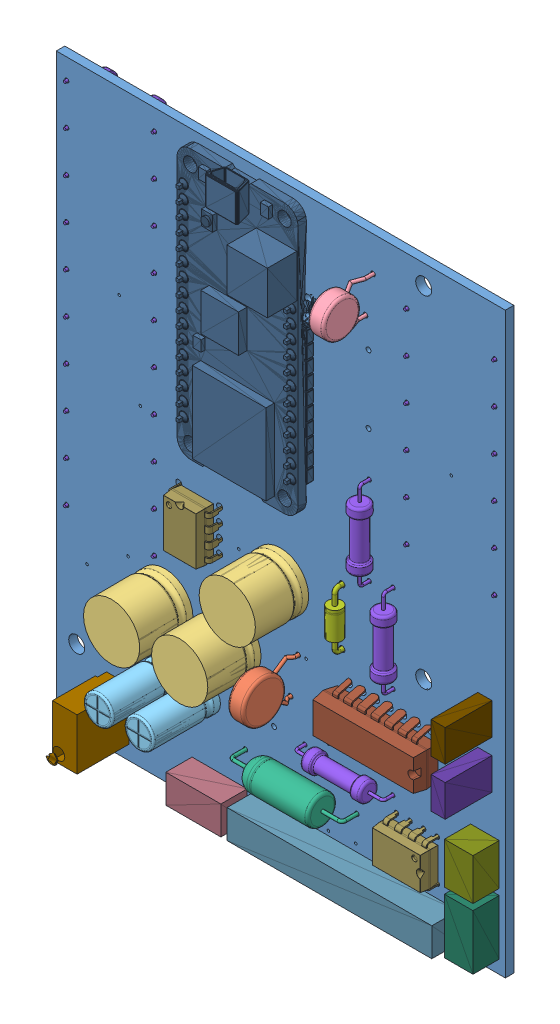
SolidWorks assembly MCB, configuration Default. Lengths in mm.
Overall size (83.82 111.16 36.76).
45 component instances, 18 part files, 0 mates.
Components (placement in the parent):
- SHEIKAHSLATE-1: SHEIKAHSLATE [Default] at origin size (83.82 111.16 36.76)
  - Board_SHEIKAHSLATE-1: Board_SHEIKAHSLATE [Default] at origin size (83.82 107.95 1.59)
  - HAU470KBAUARKR-1: HAU470KBAUARKR [Default] at (53.34 12.7 0.05) x (0 1 0) z (0 0 1) size (8 3 13.01)
  - MALREKA00DE433BG0K-1: MALREKA00DE433BG0K [Default] at (50.8 26.83 0.05) x (0 1 0) z (0 0 1) size (10.51 10.5 11.95)
  - MALREKA00DE433BG0K-2: MALREKA00DE433BG0K [Default] at (29.21 12.7 0.05) size (10.51 10.5 11.95)
  - MALREKA00DE433BG0K-3: MALREKA00DE433BG0K [Default] at (41.91 12.7 0.05) size (10.51 10.5 11.95)
  - A102J15C0GF5UAAP-1: A102J15C0GF5UAAP [Default] at (67.31 81.28 0.05) x (0 -1 0) z (0 0 1) size (7.99 3 12.01)
  - Noname_1-1: Noname_1 [Default] at (36.83 1.27 0.05) size (5.5 5.5 14.5)
  - Noname_1-2: Noname_1 [Default] at (29.21 1.27 0.05) size (5.5 5.5 14.5)
  - TVA1161-1: TVA1161 [Default] at (54.61 -3.81 0.05) size (21.4 5.51 7.51)
  - 1N5819G-1: 1N5819G [Default] at (62.23 26.67 0) x (0 -1 0) z (0 0 1) size (11.27 2.71 4.71)
  - Noname_2-1: Noname_2 [Default] at (67.31 43.18 0) x (0 -1 0) z (0 0 1) size (16.91 3.6 5.6)
  - Noname_2-2: Noname_2 [Default] at (46.99 58.42 -1.5896) x (0 1 0) z (0 0 -1) size (16.91 3.6 5.6)
  - Noname_2-3: Noname_2 [Default] at (19.05 87.63 -1.5896) x (-1 0 0) z (0 0 -1) size (16.91 3.6 5.6)
  - Noname_2-4: Noname_2 [Default] at (19.05 80.01 -1.5896) x (-1 0 0) z (0 0 -1) size (16.91 3.6 5.6)
  - Noname_2-5: Noname_2 [Default] at (19.05 72.39 -1.5896) x (-1 0 0) z (0 0 -1) size (16.91 3.6 5.6)
  - Noname_2-6: Noname_2 [Default] at (19.05 64.77 -1.5896) x (-1 0 0) z (0 0 -1) size (16.91 3.6 5.6)
  - Noname_2-7: Noname_2 [Default] at (19.05 57.15 -1.5896) x (-1 0 0) z (0 0 -1) size (16.91 3.6 5.6)
  - Noname_2-8: Noname_2 [Default] at (19.05 49.53 -1.5896) x (-1 0 0) z (0 0 -1) size (16.91 3.6 5.6)
  - Noname_2-9: Noname_2 [Default] at (19.05 41.91 -1.5896) x (-1 0 0) z (0 0 -1) size (16.91 3.6 5.6)
  - Noname_2-10: Noname_2 [Default] at (19.05 34.29 -1.5896) x (-1 0 0) z (0 0 -1) size (16.91 3.6 5.6)
  - Noname_2-11: Noname_2 [Default] at (19.05 26.67 -1.5896) x (-1 0 0) z (0 0 -1) size (16.91 3.6 5.6)
  - Noname_2-12: Noname_2 [Default] at (19.05 19.05 -1.5896) x (-1 0 0) z (0 0 -1) size (16.91 3.6 5.6)
  - Noname_2-13: Noname_2 [Default] at (82.55 44.45 -1.5896) x (1 0 0) z (0 0 -1) size (16.91 3.6 5.6)
  - Noname_2-14: Noname_2 [Default] at (82.55 52.07 -1.5896) x (1 0 0) z (0 0 -1) size (16.91 3.6 5.6)
  - Noname_2-15: Noname_2 [Default] at (82.55 59.69 -1.5896) x (1 0 0) z (0 0 -1) size (16.91 3.6 5.6)
  - Noname_2-16: Noname_2 [Default] at (82.55 67.31 -1.5896) x (1 0 0) z (0 0 -1) size (16.91 3.6 5.6)
  - Noname_2-17: Noname_2 [Default] at (82.55 74.93 -1.5896) x (1 0 0) z (0 0 -1) size (16.91 3.6 5.6)
  - Noname_2-18: Noname_2 [Default] at (82.55 82.55 -1.5896) x (1 0 0) z (0 0 -1) size (16.91 3.6 5.6)
  - Noname_2-19: Noname_2 [Default] at (48.26 78.74 -1.5896) x (0 -1 0) z (0 0 -1) size (16.91 3.6 5.6)
  - Noname_2-20: Noname_2 [Default] at (39.37 78.74 -1.5896) x (0 1 0) z (0 0 -1) size (16.91 3.6 5.6)
  - Noname_2-21: Noname_2 [Default] at (71.755 27.94 0) x (0 1 0) z (0 0 1) size (16.91 3.6 5.6)
  - Noname_2-22: Noname_2 [Default] at (39.37 58.42 -1.5896) x (0 1 0) z (0 0 -1) size (16.91 3.6 5.6)
  - Noname_2-23: Noname_2 [Default] at (63.5 2.54 0) size (16.91 3.6 5.6)
  - T93YA-1: T93YA [Default] at (20.32 -13.69 5) size (12.52 14.14 22.04)
  - Adafruit_Feather_M0_Adalogger-1: Adafruit_Feather_M0_Adalogger [Default] at (45.72 66.04 3) x (0 -1 0) z (0 0 1) size (54.99 41.16 36.76)
  - SN74HC125N-1: SN74HC125N [Default] at (71.24 12.69 0) x (-1 0 0) z (0 1 0) size (19.31 8.27 10.93)
  - DIP8-1: DIP8 [Default] at (76.2 -3.81 0) size (15.36 12.48 12.48)
  - DIP8-2: DIP8 [Default] at (35.77 29 0) x (0 1 0) z (0 0 1) size (15.36 12.48 12.48)
  - 640453-4-1: 640453-4 [Default] at (39.1318 -16.4465 0) size (10.3 5.34 4.91)
  - 1-640453-5-1: 1-640453-5 [Default] at (64.53 -16.4465 0) size (38.24 5.34 4.91)
  - 640453-4-0-1: 640453-4-0 [Default] at (92.6465 -9.1282 0) x (0 1 0) z (0 0 1) size (10.3 5.34 4.91)
  - 640453-3-1: 640453-3 [Default] at (92.6465 1.0303 0) x (-0.000018 1 0) z (0 0 1) size (7.76 5.34 4.91)
  - PPTC021LFBN-RC-1: PPTC021LFBN-RC [Default] at (88.689 15.24 0) x (0 1 0) z (0 0 1) size (5.94 2.66 8.76)
  - PPTC021LFBN-RC-1-1: PPTC021LFBN-RC-1 [Default] at (88.689 24.13 0) x (-0.000018 1 0) z (0 0 1) size (5.94 2.66 8.76)
